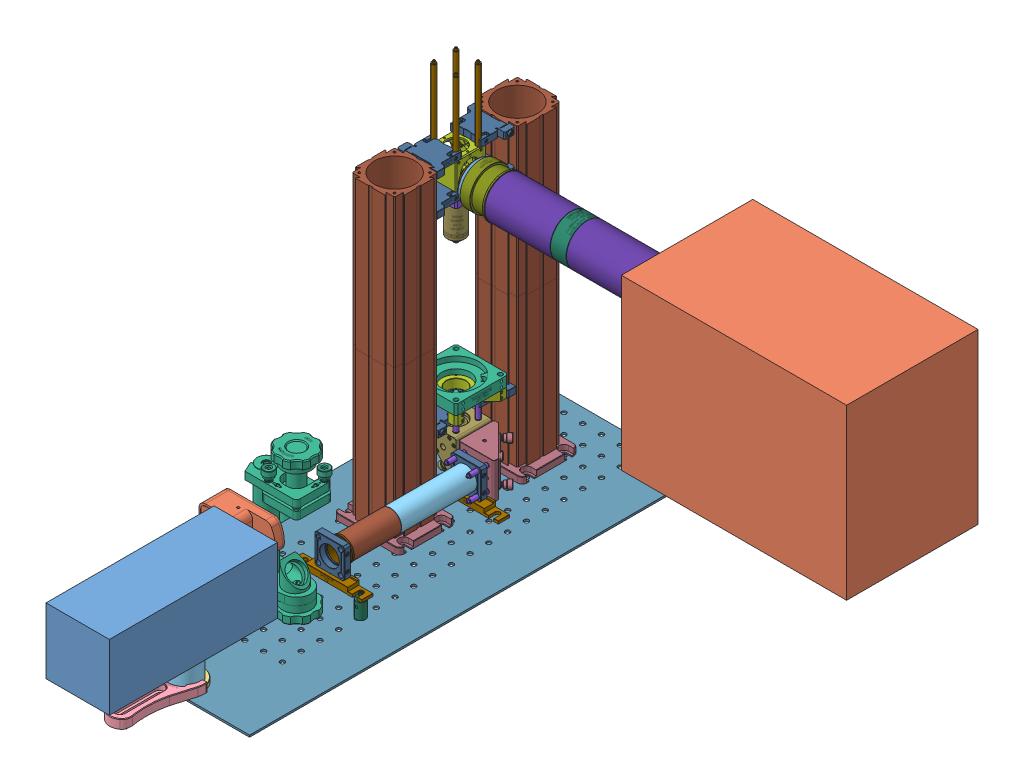
SolidWorks assembly Assembly2, configuration Default. Lengths in mm.
Overall size (719.05 492.49 737.9).
70 component instances, 37 part files, 27 mates.
Components (placement in the parent):
- Laser Sub-Assembly-1: Laser Sub-Assembly [Default] at (-416.933 -106.2176 446.3872) size (173.3 196.72 329.92)
  - Laser-1: Laser [Default] at (0 -56.1594 0) x (0 0 1) z (-1 0 0) size (238.02 88.9 85.74)
  - SH05-Solidworks-1: SH05-Solidworks [Default] at (-45.783 38.7485 -125.4012) x (0 1 0) z (0 0 -1) size (57.1 81.96 34.87)
  - PB4-Solidworks-1: PB4-Solidworks [Default] at (-1.2577 -106.9594 -33.431) size (46.99 12.7 46.99)
  - PF175-Solidworks-1: PF175-Solidworks [Default] at (3.3213 -76.677 -7.4391) size (53.49 12.2 106.17)
  - P2-Solidworks-1: P2-Solidworks [Web Part] at (-1.2577 -81.5594 -33.431) x (0.77638 0 -0.630266) z (0.630266 0 0.77638) size (37.74 50.8 37.94)
  - RS99-Solidworks-1: RS99-Solidworks [Default] at (-64.0174 -83.6665 -251.4056) x (0 0 1) z (-1 0 0) size (53.35 196.72 150.14)
- Objective Sub-Assembly-1: Objective Sub-Assembly [Default] at (-566.1965 226.5168 -25.2284) x (1 0 0) z (0 -1 0) size (89.31 242.24 499.06)
  - CM1-DCH-Solidworks-1: CM1-DCH-Solidworks [Web Assembly] at (101.1512 25.2284 64.8406) size (38.1 45.72 38.1)
  - CP16-Solidworks-1: CP16-Solidworks [Default] at (83.0447 27.4143 105.2952) size (41.22 40.64 8.89)
  - ER6-P4-Solidworks-1: ER6-P4-Solidworks [Default] at (115.9512 38.6905 22.9846) x (0.631657 -0.775248 0) z (-0.775248 -0.631657 0) size (5.99 157.48 5.99)
  - ER6-P4-Solidworks-2: ER6-P4-Solidworks [Default] at (114.7082 9.6603 22.9846) x (-0.373438 -0.927655 0) z (-0.927655 0.373438 0) size (5.99 157.48 5.99)
  - ER6-P4-Solidworks-3: ER6-P4-Solidworks [Default] at (85.1563 39.0388 22.9846) x (0.116187 -0.993227 0) z (-0.993227 -0.116187 0) size (5.99 157.48 5.99)
  - ER6-P4-Solidworks-4: ER6-P4-Solidworks [Default] at (87.3845 11.1687 27.9565) x (0.986967 -0.160923 0) z (0.160923 0.986967 0) size (5.99 157.48 5.99)
  - RCA2-Solidworks-1: RCA2-Solidworks [Default] at (87.6791 34.1856 4.2312) size (56.73 41.06 8.89)
  - RCA2-Solidworks-2: RCA2-Solidworks [Default] at (114.6233 16.2713 4.2312) x (-1 0 0) z (0 0 1) size (56.73 41.06 8.89)
  - XT66-200-Solidworks-1: XT66-200-Solidworks [Default] at origin size (66.04 66.04 200)
  - XT66-200-Solidworks-2: XT66-200-Solidworks [Default] at (0 -166.04 0) size (66.04 66.04 200)
  - N40X-NIR-Solidworks-1: N40X-NIR-Solidworks [Default] at (101.1512 25.2284 128.3406) x (0 0 1) z (-0.615109 0.788442 0) size (61.98 27.94 27.94)
  - RCA2-Solidworks-3: RCA2-Solidworks [Default] at (114.6233 16.2713 51.2212) x (-1 0 0) z (0 0 1) size (56.73 41.06 8.89)
  - RCA2-Solidworks-4: RCA2-Solidworks [Default] at (87.6791 34.1856 51.2212) size (56.73 41.06 8.89)
  - XT66-200-Solidworks-3: XT66-200-Solidworks [Default] at (0 0 199.9996) size (66.04 66.04 200)
  - XT66-200-Solidworks-4: XT66-200-Solidworks [Default] at (0 -166.04 199.9996) size (66.04 66.04 200)
  - XT66P1-Solidworks-1: XT66P1-Solidworks [Default] at (101.1639 108.2484 445.7898) x (0 -1 0) z (1 0 0) size (76.2 8.89 89.28)
  - XT66P1-Solidworks-2: XT66P1-Solidworks [Default] at (101.1385 -57.7916 445.7898) x (0 1 0) z (-1 0 0) size (76.2 8.89 89.28)
- Tank Sub-Assembly-1: Tank Sub-Assembly [Default] at origin size (492.39 222.91 245.75) (hidden)
  - WaterBath-1: WaterBath [Default] at (-614.8457 -4.3008 0) size (203.2 101.6 101.6)
  - L490-Solidworks-1: L490-Solidworks [Default] at (-624.5838 -100.8719 -9.0343) x (0 0 -1) z (1 0 0) size (245.75 83.31 101.6)
  - LX20-Solidworks-1: LX20-Solidworks [Chamfers] at (-650.9996 -116.3058 97.2581) size (132.4 38.28 116.16)
  - Opticell-1: Opticell [Default] at (-256.3578 52.6159 0) x (0.739747 0.672885 0) z (0 0 1) size (76.36 12.75 129.72)
- Camera Sub-Assembly-1: Camera Sub-Assembly [Default] at (-445.9953 152.4 0) x (0 0 1) z (-1 0 0) size (71.93 71.93 293.6)
  - SM2NFM2-Solidworks-1: SM2NFM2-Solidworks [Default] at (0 0 -280.4) x (0 1 0) z (-1 0 0) size (63.5 16.37 63.5)
  - TTL200-S8-Solidworks-1: TTL200-S8-Solidworks [Default] at (0 0 -147.2485) size (55.88 55.88 28)
  - SM2V15-Solidworks-1: SM2V15-Solidworks [Default] at (18.0496 -29.8565 -283.1388) x (0 0 -1) z (0.951776 0.306793 0) size (51.56 57.15 57.15)
  - SM2M35-Solidworks-1: SM2M35-Solidworks [Default] at (-10.7846 9.351 -214.221) x (0.99081 -0.135264 0) z (0 0 1) size (55.88 55.88 88.9)
  - SM2M35-Solidworks-2: SM2M35-Solidworks [Default] at (-11.8362 7.9783 -103.671) x (0.999895 -0.014459 0) z (0 0 1) size (55.88 55.88 88.9)
  - SM2V15-Solidworks-2: SM2V15-Solidworks [Default] at (-9.1968 -33.7176 -11.3581) x (0 0 1) z (-0.999373 0.035397 0) size (51.56 57.15 57.15)
  - SM1T2-Solidworks-1: SM1T2-Solidworks [Default] at (0 0 1.778) x (0.997143 -0.075539 0) z (0 0 1) size (31.75 31.75 12.7)
  - SM2A6-Solidworks-2: SM2A6-Solidworks [Default] at (0 0 -9.144) x (0.976828 -0.214025 0) z (0 0 1) size (51.69 51.69 5.08)
- hpvx2-1: hpvx2 [Default] at origin size (311.15 228.6 177.8)
- Small Condenser Adjustable Sub-Assembly-1: Small Condenser Adjustable Sub-Assembly [Default] at (-444.7267 -88.209 -35.56) x (0 -1 0) z (1 0 0) size (105.41 279.92 134.62)
  - LB1437-Solidworks-1: LB1437-Solidworks [Default] at (76.2 -225.5719 31.115) x (0.879994 0 -0.474985) z (0 -1 0) size (25.4 25.4 3.05)
  - LB1761-Solidworks-1: LB1761-Solidworks [Default] at (76.2 -80.7719 31.115) x (0.962182 0 -0.272406) z (0 -1 0) size (25.4 25.4 8.98)
  - SM1L40-Solidworks-1: SM1L40-Solidworks [Default] at (78.1038 -120.8912 29.0232) x (-1 0 0) z (0 1 0) size (30.48 30.48 105.41)
  - CSA1003-Solidworks-1: CSA1003-Solidworks [Default] at (47.6181 -122.449 -34.035) x (0 -1 0) z (0 0 1) size (71.12 13.97 71.12)
  - LCP02-Solidworks-1: LCP02-Solidworks [Default] at (20.32 -35.5599 -20.32) x (0 0 -1) z (1 0 0) size (70.75 70.61 12.7)
  - ER1-Solidworks-1: ER1-Solidworks [Default] at (60.5626 -51.9737 -8.2009) x (0.379624 -0.925141 0) z (-0.925141 -0.379624 0) size (5.99 30.48 5.99)
  - ER1-Solidworks-2: ER1-Solidworks [Default] at (91.197 -74.8759 17.6658) x (0.724997 0 0.688752) z (-0.688752 0 0.724997) size (5.99 30.48 5.99)
  - ER1-Solidworks-3: ER1-Solidworks [Default] at (89.6524 -50.6607 -8.2009) x (-0.638668 -0.769482 0) z (-0.769482 0.638668 0) size (5.99 30.48 5.99)
  - ER1-Solidworks-4: ER1-Solidworks [Default] at (89.737 -21.0745 -3.2291) x (-0.889374 0.45718 0) z (-0.45718 -0.889374 0) size (5.99 30.48 5.99)
  - CPB1-Solidworks-2: CPB1-Solidworks [Default] at (105.41 -246.8879 78.74) x (0 0 1) z (0 -1 0) size (95.25 10.79 15.24)
  - CP08-Solidworks-2: CP08-Solidworks [Default] at (76.2 -253.8729 31.115) x (0 0 -1) z (0 1 0) size (41.5 40.64 8.89)
  - SM1T2-Solidworks-1: SM1T2-Solidworks [Default] at (76.2 -238.5059 31.115) x (1 0 0) z (0 1 0) size (31.75 31.75 12.7)
  - SM1L25-Solidworks-1: SM1L25-Solidworks [Default] at (13.7682 -184.6239 44.6501) x (0 -1 0) z (0.940748 0 0.339105) size (67.31 30.48 30.48)
  - CPB1-Solidworks-3: CPB1-Solidworks [Default] at (105.41 -62.2299 78.74) x (0 0 1) z (0 -1 0) size (95.25 10.79 15.24)
  - CP08-Solidworks-3: CP08-Solidworks [Default] at (76.2 -69.2149 31.115) x (0 0 -1) z (0 1 0) size (41.5 40.64 8.89)
  - KCB1C-Solidworks-2: KCB1C-Solidworks [Default] at (76.2 -35.5599 -20.32) x (-1 0 0) z (0 0 1) size (51.13 48.49 51.11)
  - KCB1-Solidworks-2: KCB1-Solidworks [Default] at (52.07 -11.4299 55.245) x (0 0 -1) z (0 -1 0) size (51.13 48.26 51.1)
  - ER1-Solidworks-5: ER1-Solidworks [Default] at (59.6581 -74.8759 16.2812) x (-0.605509 0 0.795839) z (-0.795839 0 -0.605509) size (5.99 30.48 5.99)
  - ER1-Solidworks-6: ER1-Solidworks [Default] at (59.6581 -20.7263 -8.2009) x (-0.605478 -0.795862 0) z (-0.795862 0.605478 0) size (5.99 30.48 5.99)
  - ER1-Solidworks-7: ER1-Solidworks [Default] at (61.2205 -69.904 44.5643) x (0.735372 0 -0.677663) z (-0.677663 0 -0.735372) size (5.99 30.48 5.99)
  - ER1-Solidworks-8: ER1-Solidworks [Default] at (90.5171 -69.904 44.7226) x (0.349448 0 -0.936956) z (-0.936956 0 -0.349448) size (5.99 30.48 5.99)
  - ER1-Solidworks-9: ER1-Solidworks [Default] at (41.8559 -51.8424 -4.448) x (0 -0.159937 0.987127) z (0 -0.987127 -0.159937) size (5.99 30.48 5.99)
  - ER1-Solidworks-10: ER1-Solidworks [Default] at (41.8559 -51.2056 -36.73) x (0 -0.946564 -0.322515) z (0 0.322515 -0.946564) size (5.99 30.48 5.99)
  - ER1-Solidworks-11: ER1-Solidworks [Default] at (36.8841 -19.2252 -34.5304) x (0 0.22178 0.975097) z (0 0.975097 -0.22178) size (5.99 30.48 5.99)
  - ER1-Solidworks-12: ER1-Solidworks [Default] at (36.8841 -19.4762 -6.4293) x (0 0.999873 0.015911) z (0 0.015911 -0.999873) size (5.99 30.48 5.99)
  - RCA2-Solidworks-1: RCA2-Solidworks [Default] at (68.2294 -44.5171 -6.8478) x (0 0 -1) z (-1 0 0) size (56.73 41.06 8.89)
  - RCA2-Solidworks-2: RCA2-Solidworks [Default] at (68.2294 -26.6027 -33.7921) x (0 0 1) z (-1 0 0) size (56.73 41.06 8.89)
- Table-1: Table [Default] at (-465.0453 -221.559 0) x (0 0 1) z (-1 0 0) size (609.6 2.54 254)
- TR1-Solidworks-1: TR1-Solidworks [Default] at (-375.5117 -219.019 218.313) size (12.67 29.6 12.87)
Mates (geometry in assembly coordinates):
- Concentric3: concentric anti-aligned: circle of ?; circle of ?
- Concentric4: concentric anti-aligned: circle of Objective Sub-Assembly-1/CM1-DCH-Solidworks-1; circle of ?
- Coincident9: coincident anti-aligned: plane of Objective Sub-Assembly-1/CM1-DCH-Solidworks-1 through (-479.704 133.35 19.05) normal (1 0 0); plane of ? through (-479.704 173.8331 -17.9239) normal (-1 0 0)
- Concentric5: concentric anti-aligned: cylinder of Camera Sub-Assembly-1/SM2M35-Solidworks-1 through (-240.9318 152.4 0) axis (-1 0 0) radius 27.94; cylinder of hpvx2-1 through (-152.4 152.4 0) axis (1 0 0) radius 29.1375
- Coincident10: coincident anti-aligned: plane of Camera Sub-Assembly-1/SM2NFM2-Solidworks-1 through (-158.75 152.4547 -0.0457) normal (1 0 0); plane of hpvx2-1 through (-158.75 152.4 0) normal (-1 0 0)
- Coincident13: coordinate: point of hpvx2-1; point of assembly
- Parallel10: parallel anti-aligned: plane of hpvx2-1 through (0 228.6 0) normal (0 1 0); plane of ? through (-473.3553 -219.019 -28.5749) normal (0 -1 0)
- Parallel11: parallel aligned: plane of hpvx2-1 through (152.4 228.6 88.9) normal (1 0 0); plane of Small Condenser Adjustable Sub-Assembly-1/CSA1003-Solidworks-1 through (-429.4866 -88.209 -35.56) normal (1 0 0)
- Concentric6: concentric anti-aligned: circle of ?; circle of Small Condenser Adjustable Sub-Assembly-1/CSA1003-Solidworks-1
- Parallel12: parallel anti-aligned: plane of hpvx2-1 through (152.4 228.6 88.9) normal (1 0 0); plane of Table-1 through (-566.6453 -219.019 -177.8) normal (-1 0 0)
- Coincident19: coincident aligned: plane of Table-1 through (-465.0453 -221.559 0) normal (0 0 1); plane of assembly through (0 0 0) normal (0 0 1)
- Coincident20: coincident aligned: plane of Objective Sub-Assembly-1/XT66-200-Solidworks-1 through (-465.0453 226.5168 -25.2284) normal (-1 0 0); plane of Table-1 through (-465.0453 -221.559 0) normal (-1 0 0)
- Coincident21: coincident anti-aligned: plane of Objective Sub-Assembly-1/XT66P1-Solidworks-1 through (-449.1576 -219.019 67.145) normal (0 -1 0); plane of Table-1 through (-465.0453 -219.019 0) normal (0 1 0)
- Coincident22: coincident anti-aligned: plane of ? through (-473.3553 -219.019 -28.5749) normal (0 -1 0); plane of Table-1 through (-498.7541 -219.019 0) normal (0 1 0)
- Coincident23: coincident aligned: plane of Tank Sub-Assembly-1/WaterBath-1 through (-614.8457 -4.3008 0) normal (0 0 1); plane of assembly through (0 0 0) normal (0 0 1)
- Concentric9: concentric anti-aligned: circle of Small Condenser Adjustable Sub-Assembly-1/CPB1-Solidworks-2; circle of TR1-Solidworks-1
- Coincident35: coincident anti-aligned: plane of Table-1 through (-465.0453 -219.019 0) normal (0 1 0); plane of TR1-Solidworks-1 through (-369.6824 -219.019 218.313) normal (0 -1 0)
- Coincident38: coincident anti-aligned: plane of Small Condenser Adjustable Sub-Assembly-1/CPB1-Solidworks-2 through (-461.2367 -193.619 211.328) normal (0 -1 0); plane of TR1-Solidworks-1 through (-375.5117 -193.619 218.313) normal (0 1 0)
- Parallel15: parallel aligned: plane of Laser Sub-Assembly-1/Laser-1 through (-416.933 -162.377 446.3872) normal (0 -1 0); plane of Objective Sub-Assembly-1/XT66-200-Solidworks-2 through (-435.9369 -10.3834 -100.4861) normal (0 -1 0)
- Parallel16: parallel aligned: plane of Laser Sub-Assembly-1/Laser-1 through (-416.933 -73.477 446.3872) normal (0 1 0); plane of hpvx2-1 through (0 228.6 0) normal (0 1 0)
- Parallel17: parallel aligned: plane of Laser Sub-Assembly-1/Laser-1 through (-416.933 -73.477 446.3872) normal (0 1 0); plane of Tank Sub-Assembly-1/L490-Solidworks-1 through (-564.0457 -4.3008 -50.8) normal (0 1 0)
- Coincident40: coincident anti-aligned: plane of Table-1 through (-465.0453 -219.019 0) normal (0 1 0); plane of Laser Sub-Assembly-1/PF175-Solidworks-1 through (-418.1907 -219.019 499.6912) normal (0 -1 0)
- Coincident41: coincident anti-aligned: plane of Laser Sub-Assembly-1/PF175-Solidworks-1 through (-413.6117 -182.8946 438.9481) normal (1 0 0); plane of assembly through (-413.6117 0 0) normal (-1 0 0)
- Coincident42: coincident anti-aligned: plane of Table-1 through (-465.0453 -219.019 0) normal (0 1 0); circle of Laser Sub-Assembly-1/RS99-Solidworks-1
- Distance2: distance = 6.35 mm anti-aligned: plane of Laser Sub-Assembly-1/RS99-Solidworks-1 through (-458.5659 -196.7925 232.918) normal (0 0 -1); plane of Small Condenser Adjustable Sub-Assembly-1/CPB1-Solidworks-2 through (-461.2367 -193.619 226.568) normal (0 0 1)
- Coincident43: coincident anti-aligned: plane of Objective Sub-Assembly-1/CM1-DCH-Solidworks-1 through (-445.9953 133.35 19.05) normal (1 0 0); plane of Camera Sub-Assembly-1/SM1T2-Solidworks-1 through (-445.9953 160.3026 11.0493) normal (-1 0 0)
- Coincident44: coincident aligned: plane of Camera Sub-Assembly-1 through (-445.9953 152.4 0) normal (0 0 1); plane of assembly
